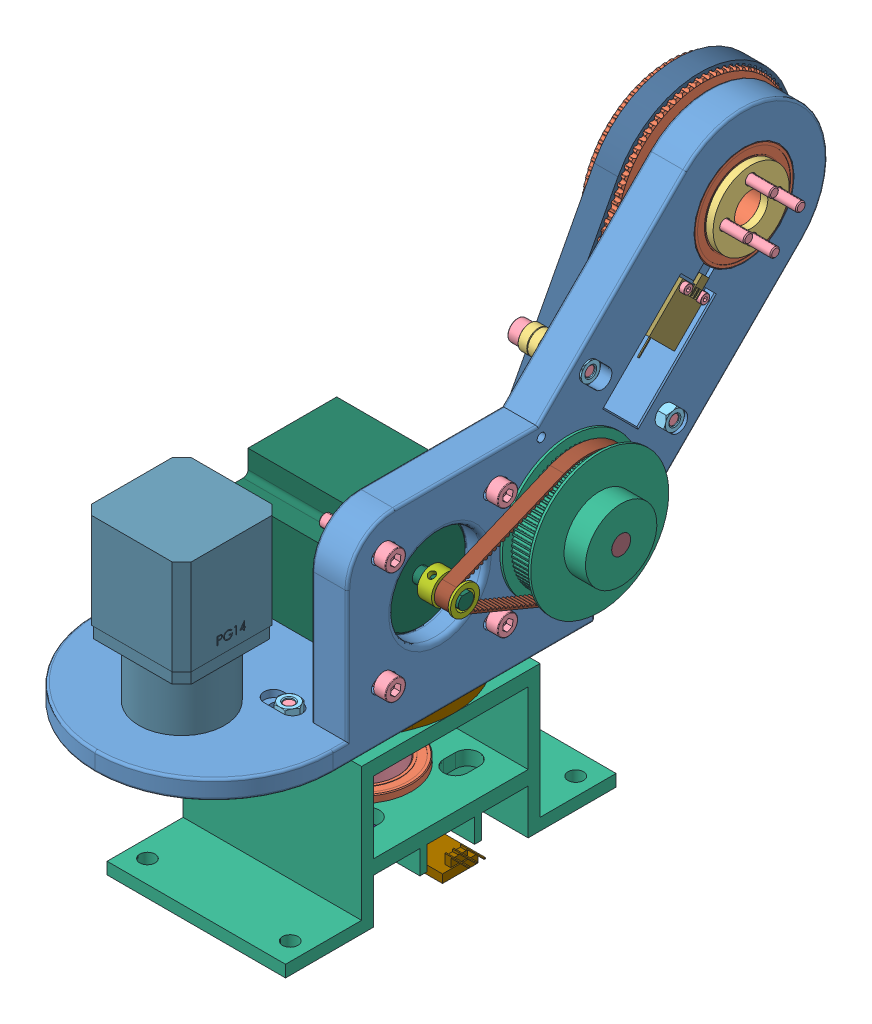
SolidWorks assembly arm1, configuration Default. Lengths in mm.
Overall size (123.1 252.71 277.96).
84 component instances, 27 part files, 181 mates.
Components (placement in the parent):
- arm1-1: arm1 [Default] at (0 22.25 32) x (0 0 1) z (0 1 0) size (257.74 100 155.28)
- PulleyHtd3m80Tbore8-2: PulleyHtd3m80Tbore8 [Default] at (25.5 142.4912 -110.7437) x (0 -0.999796 -0.020218) z (1 0 0) size (75.96 75.93 32)
- bearingCover-1: bearingCover [Default] at (50 142.4912 -110.7437) x (0 -0.999796 -0.020218) z (1 0 0) size (32 32 3)
- shaftJ1-1: shaftJ1 [Default] at (0 -34.75 0) x (0 0 -1) z (1 0 0) size (50 69 50)
- Pulleyhtd3m20Tbore8-1: Pulleyhtd3m20Tbore8 [Default] at (0 12.5 75.6) x (1 0 0) z (0 -1 0) size (22 22 24)
- pulley2GT80T-1: pulley2GT80T [Default] at (57.6 67.75 -36.0025) x (0 -0.778145 -0.628085) z (1 0 0) size (58 58 22)
- pulley2GT16Tbore6.35-1: pulley2GT16Tbore6.35 [Default] at (56.1 67.75 17.0975) x (0 0.483708 -0.87523) z (1 0 0) size (12.2 12.2 14)
- PulleyHTD3m15Tbore8-1: PulleyHTD3m15Tbore8 [Default] at (26.5 67.75 -36.0025) x (0 0.57686 0.816843) z (1 0 0) size (14 14 19.5)
- BeltHTD3m312L20T80T-1: BeltHTD3m312L20T80T [Default] at (0 12.5 0) x (0 0 1) z (0 1 0) size (125.04 78.09 10)
- BeltHTD3m363L15T80T-1: BeltHTD3m363L15T80T [Default] at (26.5 142.4912 -110.7437) x (0 -0.707107 0.707107) z (-1 0 0) size (152.76 78.09 10)
- belt2GT210L-1: belt2GT210L [Default] at (56.1 67.75 17.0975) x (0 0 -1) z (1 0 0) size (84.41 51.68 6)
- MagneticSensorV2-2: MagneticSensorV2 [Default] at (45.9 115.6211 -83.8737) x (0 -0.707107 0.707107) z (1 0 0) size (31 15 9)
- shaft8x70-1: shaft8x70 [Default] at (73.1 67.75 -36.0025) x (0 0 1) z (-1 0 0) size (8 8 61)
- Nema17L40PG14-1: Nema17L40PG14 [Default] at (0 99.75 75.6) x (0 0 -1) z (0 -1 0) size (42 42 88.5)
- Nema23_57x57x56-2: Nema23_57x57x56 [Default] at (-12 67.75 17.0975) x (0 0 -1) z (1 0 0) size (57 57 73)
- BeltTensionSpacer-1: BeltTensionSpacer [Default] at (35 113.7119 -46.6091) x (0 -0.41678 -0.909008) z (-1 0 0) size (6.4 6.4 3)
- BeltTensionSpacer-2: BeltTensionSpacer [Default] at (35 78.3566 -81.9645) x (0 -0.41678 -0.909008) z (-1 0 0) size (6.4 6.4 3)
- BeltTensionSpacer-6: BeltTensionSpacer [Default] at (-24.5 19.25 55) x (0.999608 0 0.027999) z (0 1 0) size (6.4 6.4 3)
- BeltTensionSpacer-5: BeltTensionSpacer [Default] at (24.5 22.25 55) x (0.852155 0 0.52329) z (0 -1 0) size (6.4 6.4 3)
- Washer45x60x1-2: Washer45x60x1 [5909K79] at (0 22.25 0) x (0 -1 0) z (0.730209 0 -0.683224) size (1 65 65)
- Washer45x60x1-1: Washer45x60x1 [5909K79] at (0 18.3 0) x (0 -1 0) z (0.528749 0 -0.848778) size (1 65 65)
- NeedleThrustBearing5909_45x60x3-1: NeedleThrustBearing5909_45x60x3 [5909K19] at (0 20.275 0) x (0.862783 0 0.505574) z (0.505574 0 -0.862783) size (65 3 65)
- bearing608 8x22x7-1: bearing608 8x22x7 [Default] at (50 67.75 -36.0025) x (0 -0.065699 -0.997839) z (0 0.997839 -0.065699) size (22 7 22)
- bearing608 8x22x7-2: bearing608 8x22x7 [Default] at (35 67.75 -36.0025) x (0 -0.995759 -0.092005) z (0 -0.092005 0.995759) size (22 7 22)
- bearing6806 30x42x7-3: bearing6806 30x42x7 [5972K282] at (38.5 142.4912 -110.7437) x (0 0.778145 0.628085) z (1 0 0) size (42 42 7)
- bearing6806 30x42x7-4: bearing6806 30x42x7 [5972K282] at (46.5 142.4912 -110.7437) x (0 -0.232241 -0.972658) z (-1 0 0) size (42 42 7)
- Bearing105 5x10x4-1: Bearing105 5x10x4 [7804K106] at (30 113.7119 -46.6091) x (0 0.558787 -0.829311) z (-1 0 0) size (10 10 4)
- Bearing105 5x10x4-4: Bearing105 5x10x4 [7804K106] at (26.1 78.3566 -81.9645) x (0 -0.623411 0.781894) z (-1 0 0) size (10 10 4)
- Bearing105 5x10x4-9: Bearing105 5x10x4 [7804K106] at (24.5 17.25 55) x (0.890608 0 -0.454771) z (0 -1 0) size (10 10 4)
- Bearing105 5x10x4-10: Bearing105 5x10x4 [7804K106] at (24.5 13.25 55) x (0.890608 0 -0.454771) z (0 -1 0) size (10 10 4)
- Bearing105 5x10x4-11: Bearing105 5x10x4 [7804K106] at (-24.5 13.25 55) x (-0.374722 0 0.927137) z (0 1 0) size (10 10 4)
- Bearing105 5x10x4-12: Bearing105 5x10x4 [7804K106] at (-24.5 17.25 55) x (0.156116 0 0.987739) z (0 1 0) size (10 10 4)
- Bearing105 5x10x4-2: Bearing105 5x10x4 [7804K106] at (26 113.7119 -46.6091) x (0 -0.774653 -0.632387) z (-1 0 0) size (10 10 4)
- Bearing105 5x10x4-3: Bearing105 5x10x4 [7804K106] at (30.1 78.3566 -81.9645) x (0 -0.931032 -0.364937) z (1 0 0) size (10 10 4)
- socket head cap screw_iso-13: socket head cap screw_iso [ISO 4762 M4 x 12 - 12N] at (0 38.25 20) x (0 -1 0) z (0 0 1) size (16 7 7)
- socket head cap screw_iso-14: socket head cap screw_iso [ISO 4762 M4 x 12 - 12N] at (20 38.25 0) x (0 -1 0) z (0 0 1) size (16 7 7)
- socket head cap screw_iso-15: socket head cap screw_iso [ISO 4762 M4 x 12 - 12N] at (0 38.25 -20) x (0 -1 0) z (0 0 1) size (16 7 7)
- socket head cap screw_iso-16: socket head cap screw_iso [ISO 4762 M4 x 12 - 12N] at (-20 38.25 0) x (0 -1 0) z (0 0 1) size (16 7 7)
- hex nut style 1 gradeab_iso-1: hex nut style 1 gradeab_iso [ISO - 4032 - M5 - W - N] at (49.7 113.7119 -46.6091) x (0 -0.707107 0.707107) z (1 0 0) size (8 9.24 4.7)
- hex nut style 1 gradeab_iso-2: hex nut style 1 gradeab_iso [ISO - 4032 - M5 - W - N] at (49.7 78.3566 -81.9645) x (0 0.965926 0.258819) z (1 0 0) size (8 9.24 4.7)
- socket head cap screw_iso-20: socket head cap screw_iso [ISO 4762 M5 x 25 - 25N] at (19 113.7119 -46.6091) size (30 8.5 8.5)
- socket head cap screw_iso-21: socket head cap screw_iso [ISO 4762 M5 x 25 - 25N] at (19.1 78.3566 -81.9645) size (30 8.5 8.5)
- socket head cap screw_iso-57: socket head cap screw_iso [ISO 4762 M5 x 20 - 20N] at (24.5 6.25 55) x (0 1 0) z (0 0 1) size (25 8.5 8.5)
- socket head cap screw_iso-58: socket head cap screw_iso [ISO 4762 M5 x 20 - 20N] at (-24.5 6.25 55) x (0 1 0) z (0 0 1) size (25 8.5 8.5)
- hex nut style 1 gradeab_iso-15: hex nut style 1 gradeab_iso [ISO - 4032 - M5 - W - N] at (-24.5 31.95 55) x (-0.866025 0 0.5) z (0 1 0) size (8 9.24 4.7)
- hex nut style 1 gradeab_iso-16: hex nut style 1 gradeab_iso [ISO - 4032 - M5 - W - N] at (24.5 31.95 55) x (-0.866025 0 -0.5) z (0 1 0) size (8 9.24 4.7)
- socket head cap screw_iso-63: socket head cap screw_iso [ISO 4762 M4 x 40 - 20N] at (19 153.4889 -110.5213) size (44 7 7)
- socket head cap screw_iso-64: socket head cap screw_iso [ISO 4762 M4 x 40 - 20N] at (19 142.7136 -121.7415) size (44 7 7)
- socket head cap screw_iso-65: socket head cap screw_iso [ISO 4762 M4 x 40 - 20N] at (19 131.4934 -110.9661) size (44 7 7)
- socket head cap screw_iso-66: socket head cap screw_iso [ISO 4762 M4 x 40 - 20N] at (19 142.2688 -99.746) size (44 7 7)
- socket head cap screw_iso-80: socket head cap screw_iso [ISO 4762 M2 x 12 - 12N] at (51.4 117.7424 -93.066) x (-1 0 0) z (0 0.924225 0.381849) size (14 3.8 3.8)
- socket head cap screw_iso-81: socket head cap screw_iso [ISO 4762 M2 x 12 - 12N] at (51.4 124.8135 -85.995) x (-1 0 0) z (0 0.924225 0.381849) size (14 3.8 3.8)
- hex nut style 1 gradeab_iso-25: hex nut style 1 gradeab_iso [ISO - 4032 - M2 - W - N] at (37.4 117.7424 -93.066) x (0 0 1) z (-1 0 0) size (4 4.62 1.6)
- hex nut style 1 gradeab_iso-26: hex nut style 1 gradeab_iso [ISO - 4032 - M2 - W - N] at (37.4 124.8135 -85.995) x (0 0 1) z (-1 0 0) size (4 4.62 1.6)
- socket head cap screw_iso-96: socket head cap screw_iso [ISO 4762 M5 x 25 - 25N] at (55 91.32 40.6675) x (-1 0 0) z (0 -0.924225 -0.381849) size (30 8.5 8.5)
- socket head cap screw_iso-97: socket head cap screw_iso [ISO 4762 M5 x 25 - 25N] at (55 91.32 -6.4725) x (-1 0 0) z (0 -0.924225 -0.381849) size (30 8.5 8.5)
- socket head cap screw_iso-98: socket head cap screw_iso [ISO 4762 M5 x 25 - 25N] at (55 44.18 -6.4725) x (-1 0 0) z (0 -0.924225 -0.381849) size (30 8.5 8.5)
- socket head cap screw_iso-99: socket head cap screw_iso [ISO 4762 M5 x 25 - 25N] at (55 44.18 40.6675) x (-1 0 0) z (0 -0.924225 -0.381849) size (30 8.5 8.5)
- socket head cap screw_iso-104: socket head cap screw_iso [ISO 4762 M3 x 12 - 12N] at (9.8995 19.25 85.4995) x (0 1 0) z (0 0 1) size (15 5.5 5.5)
- socket head cap screw_iso-105: socket head cap screw_iso [ISO 4762 M3 x 12 - 12N] at (9.8995 19.25 65.7005) x (0 1 0) z (0 0 1) size (15 5.5 5.5)
- socket head cap screw_iso-106: socket head cap screw_iso [ISO 4762 M3 x 12 - 12N] at (-9.8995 19.25 85.4995) x (0 1 0) z (0 0 1) size (15 5.5 5.5)
- socket head cap screw_iso-107: socket head cap screw_iso [ISO 4762 M3 x 12 - 12N] at (-9.8995 19.25 65.7005) x (0 1 0) z (0 0 1) size (15 5.5 5.5)
- hex nut style 1 gradeab_iso-35: hex nut style 1 gradeab_iso [ISO - 4032 - M5 - W - N] at (30.3 91.32 40.6675) x (0 0 1) z (-1 0 0) size (8 9.24 4.7)
- hex nut style 1 gradeab_iso-36: hex nut style 1 gradeab_iso [ISO - 4032 - M5 - W - N] at (30.3 91.32 -6.4725) x (0 0 1) z (-1 0 0) size (8 9.24 4.7)
- hex nut style 1 gradeab_iso-37: hex nut style 1 gradeab_iso [ISO - 4032 - M5 - W - N] at (30.3 44.18 -6.4725) x (0 0 1) z (-1 0 0) size (8 9.24 4.7)
- hex nut style 1 gradeab_iso-38: hex nut style 1 gradeab_iso [ISO - 4032 - M5 - W - N] at (40.3966 44.18 40.6675) x (0 0 -1) z (1 0 0) size (8 9.24 4.7)
- base-1: base [Default] x (1 0 0) z (0 1 0) size (75 138.93 61)
- bearing6806 30x42x7-1: bearing6806 30x42x7 [5972K282] at (0 -30.5984 0) x (0.837169 0 0.546944) z (0 -1 0) size (42 42 7)
- pulleyHTD3m80Tbase-1: pulleyHTD3m80Tbase [Default] at (0 12 0) x (1 0 0) z (0 1 0) size (75.63 75.63 12)
- bearing6806 30x42x7-2: bearing6806 30x42x7 [5972K282] at (0 14.3 0) x (0.999895 0 -0.014508) z (0 1 0) size (42 42 7)
- shaftJ1endPlate-1: shaftJ1endPlate [Default] at (0 -34.75 0) x (0 0 -1) z (0 -1 0) size (40 40 6)
- MagneticSensor-3: MagneticSensor [Default] at (31.5 -49.5984 0) x (1 0 0) z (0 1 0) size (31 15 7.5)
- socket head cap screw_iso-132: socket head cap screw_iso [ISO 4762 M5 x 16 - 16N] at (21 -5 -21) x (0 1 0) z (0 0 1) size (21 8.5 8.5)
- socket head cap screw_iso-133: socket head cap screw_iso [ISO 4762 M5 x 16 - 16N] at (21 -5 21) x (0 1 0) z (0 0 1) size (21 8.5 8.5)
- socket head cap screw_iso-134: socket head cap screw_iso [ISO 4762 M5 x 16 - 16N] at (-21 -5 21) x (0 1 0) z (0 0 1) size (21 8.5 8.5)
- socket head cap screw_iso-135: socket head cap screw_iso [ISO 4762 M5 x 16 - 16N] at (-21 -5 -21) x (0 1 0) z (0 0 1) size (21 8.5 8.5)
- socket head cap screw_iso-136: socket head cap screw_iso [ISO 4762 M3 x 16 - 16N] at (12.5 -43.75 0) x (0 1 0) z (0 0 1) size (19 5.5 5.5)
- socket head cap screw_iso-137: socket head cap screw_iso [ISO 4762 M3 x 16 - 16N] at (0 -43.75 12.5) x (0 1 0) z (0 0 1) size (19 5.5 5.5)
- socket head cap screw_iso-138: socket head cap screw_iso [ISO 4762 M3 x 16 - 16N] at (-12.5 -43.75 0) x (0 1 0) z (0 0 1) size (19 5.5 5.5)
- socket head cap screw_iso-139: socket head cap screw_iso [ISO 4762 M3 x 16 - 16N] at (0 -43.75 -12.5) x (0 1 0) z (0 0 1) size (19 5.5 5.5)
- socket head cap screw_iso-140: socket head cap screw_iso [ISO 4762 M2 x 12 - 12N] at (23.5 -51.5984 -5) x (0 1 0) z (-0.11823 0 0.992986) size (14 3.8 3.8)
- socket head cap screw_iso-141: socket head cap screw_iso [ISO 4762 M2 x 12 - 12N] at (23.5 -51.5984 5) x (0 1 0) z (0 0 1) size (14 3.8 3.8)
- hex nut style 1 gradeab_iso-59: hex nut style 1 gradeab_iso [ISO - 4032 - M2 - W - N] at (23.5 -40.9984 -5) x (1 0 0) z (0 1 0) size (4 4.62 1.6)
- hex nut style 1 gradeab_iso-60: hex nut style 1 gradeab_iso [ISO - 4032 - M2 - W - N] at (23.5 -40.9984 5) x (1 0 0) z (0 1 0) size (4 4.62 1.6)
Mates (geometry in assembly coordinates):
- Fix J1: parallel aligned: plane of base-1 through (37.5 6 37.5) normal (1 0 0); plane of arm1-1 through (50 30.25 -48) normal (1 0 0)
- Concentric1: concentric aligned: cylinder of base-1 through (0 29.44 0) axis (0 -1 0) radius 21.05; cylinder of bearing6806 30x42x7-1 through (0 -34.0984 0) axis (0 -1 0) radius 21
- Coincident1: coincident anti-aligned: plane of base-1 through (0 -34.0984 0) normal (0 1 0); plane of bearing6806 30x42x7-1 through (-11.2944 -34.0984 17.2875) normal (0 -1 0)
- Concentric2: concentric anti-aligned: cylinder of base-1 through (0 6 0) axis (0 -1 0) radius 16; cylinder of pulleyHTD3m80Tbase-1 through (0 10.8 0) axis (0 1 0) radius 21.05
- Concentric3: concentric anti-aligned: cylinder of base-1 through (21 6 21) axis (0 -1 0) radius 2.75; cylinder of pulleyHTD3m80Tbase-1 through (21 6 21) axis (0 1 0) radius 3
- Coincident2: coincident anti-aligned: plane of base-1 through (0 6 0) normal (0 1 0); plane of pulleyHTD3m80Tbase-1 through (0 6 0) normal (0 -1 0)
- Concentric4: concentric aligned: cylinder of base-1 through (21 6 -21) axis (0 -1 0) radius 2.75; cylinder of socket head cap screw_iso-132 through (21 -36.75 -21) axis (0 -1 0) radius 4.25
- Coincident3: coincident anti-aligned: plane of base-1 through (0 0 0) normal (0 -1 0); plane of socket head cap screw_iso-132 through (16.75 0 -21) normal (0 1 0)
- Concentric5: concentric aligned: cylinder of base-1 through (21 6 21) axis (0 -1 0) radius 2.75; cylinder of socket head cap screw_iso-133 through (21 -36.75 21) axis (0 -1 0) radius 4.25
- Coincident4: coincident anti-aligned: plane of base-1 through (0 0 0) normal (0 -1 0); plane of socket head cap screw_iso-133 through (16.75 0 21) normal (0 1 0)
- Concentric6: concentric aligned: cylinder of base-1 through (-21 6 21) axis (0 -1 0) radius 2.75; cylinder of socket head cap screw_iso-134 through (-21 -36.75 21) axis (0 -1 0) radius 4.25
- Coincident5: coincident anti-aligned: plane of base-1 through (0 0 0) normal (0 -1 0); plane of socket head cap screw_iso-134 through (-25.25 0 21) normal (0 1 0)
- Concentric7: concentric aligned: cylinder of base-1 through (-21 6 -21) axis (0 -1 0) radius 2.75; cylinder of socket head cap screw_iso-135 through (-21 -36.75 -21) axis (0 -1 0) radius 4.25
- Coincident6: coincident anti-aligned: plane of base-1 through (0 0 0) normal (0 -1 0); plane of socket head cap screw_iso-135 through (-25.25 0 -21) normal (0 1 0)
- Concentric8: concentric aligned: cylinder of pulleyHTD3m80Tbase-1 through (0 10.8 0) axis (0 1 0) radius 21.05; cylinder of bearing6806 30x42x7-2 through (0 17.8 0) axis (0 1 0) radius 21
- Coincident7: coincident anti-aligned: plane of pulleyHTD3m80Tbase-1 through (0 10.8 0) normal (0 1 0); plane of bearing6806 30x42x7-2 through (-0.2996 10.8 -20.6478) normal (0 -1 0)
- Concentric9: concentric aligned: cylinder of pulleyHTD3m80Tbase-1 through (0 10.8 0) axis (0 1 0) radius 21.05; cylinder of Washer45x60x1-1 through (0 17.8 0) axis (0 1 0) radius 32.5
- Coincident8: coincident anti-aligned: plane of pulleyHTD3m80Tbase-1 through (0 17.8 0) normal (0 1 0); plane of Washer45x60x1-1 through (0 17.8 0) normal (0 -1 0)
- Concentric10: concentric anti-aligned: cylinder of pulleyHTD3m80Tbase-1 through (0 10.8 0) axis (0 1 0) radius 21.05; cylinder of NeedleThrustBearing5909_45x60x3-1 through (0 18.775 0) axis (0 -1 0) radius 32.5
- Distance1: distance = 0.2 mm anti-aligned: plane of NeedleThrustBearing5909_45x60x3-1 through (-16.4311 19 28.0405) normal (0 -1 0); plane of Washer45x60x1-1 through (0 18.8 0) normal (0 1 0)
- Concentric11: concentric aligned: cylinder of pulleyHTD3m80Tbase-1 through (0 10.8 0) axis (0 1 0) radius 21.05; cylinder of Washer45x60x1-2 through (0 21.75 0) axis (0 1 0) radius 22.525
- Distance2: distance = 0.2 mm anti-aligned: plane of NeedleThrustBearing5909_45x60x3-1 through (-16.2626 21.55 27.7529) normal (0 1 0); plane of Washer45x60x1-2 through (0 21.75 0) normal (0 -1 0)
- Concentric12: concentric aligned: cylinder of base-1 through (0 6 0) axis (0 -1 0) radius 16; cylinder of arm1-1 through (0 30.25 0) axis (0 -1 0) radius 15.5
- Coincident12: coincident anti-aligned: plane of arm1-1 through (0 22.75 0) normal (0 -1 0); plane of Washer45x60x1-2 through (0 22.75 0) normal (0 1 0)
- Concentric15: concentric anti-aligned: cylinder of arm1-1 through (0 30.25 75.6) axis (0 -1 0) radius 11.5; cylinder of Nema17L40PG14-1 through (0 30.25 75.6) axis (0 1 0) radius 18
- Concentric16: concentric aligned: cylinder of arm1-1 through (-9.8995 30.25 85.4995) axis (0 -1 0) radius 1.65; cylinder of Nema17L40PG14-1 through (-9.8995 38.25 85.4995) axis (0 -1 0) radius 2
- Coincident16: coincident anti-aligned: plane of arm1-1 through (0 30.25 32) normal (0 1 0); plane of Nema17L40PG14-1 through (0 30.25 75.6) normal (0 -1 0)
- Concentric20: concentric anti-aligned: cylinder of Nema17L40PG14-1 through (0 11.25 75.6) axis (0 1 0) radius 4; cylinder of Pulleyhtd3m20Tbore8-1 through (0 30 75.6) axis (0 -1 0) radius 11
- Coincident17: coincident anti-aligned: plane of pulleyHTD3m80Tbase-1 through (0 18 0) normal (0 1 0); plane of Pulleyhtd3m20Tbore8-1 through (0 18 75.6) normal (0 -1 0)
- Concentric21: concentric aligned: cylinder of NeedleThrustBearing5909_45x60x3-1 through (0 18.775 0) axis (0 -1 0) radius 32.5; cylinder of BeltHTD3m312L20T80T-1 through (0 17.5 0) axis (0 -1 0) radius 39.0462
- Concentric22: concentric aligned: cylinder of Pulleyhtd3m20Tbore8-1 through (0 30 75.6) axis (0 -1 0) radius 11; cylinder of BeltHTD3m312L20T80T-1 through (0 17.5 75.6) axis (0 -1 0) radius 10.3983
- Distance3: distance = 0.5 mm anti-aligned: plane of Pulleyhtd3m20Tbore8-1 through (0 18 75.6) normal (0 -1 0); plane of BeltHTD3m312L20T80T-1 through (0 17.5 0) normal (0 1 0)
- Concentric23: concentric aligned: cylinder of arm1-1 through (0 30.25 0) axis (0 -1 0) radius 15.5; cylinder of shaftJ1-1 through (0 30.25 0) axis (0 -1 0) radius 15
- Concentric24: concentric aligned: cylinder of arm1-1 through (0 30.25 20) axis (0 -1 0) radius 2.75; cylinder of shaftJ1-1 through (0 34.25 20) axis (0 -1 0) radius 2.25
- Coincident19: coincident anti-aligned: plane of arm1-1 through (0 30.25 32) normal (0 1 0); plane of shaftJ1-1 through (0 30.25 0) normal (0 -1 0)
- Coincident24: coincident anti-aligned: plane of shaftJ1-1 through (0 -34.75 0) normal (0 -1 0); plane of shaftJ1endPlate-1 through (0 -34.75 0) normal (0 1 0)
- Concentric29: concentric anti-aligned: cylinder of shaftJ1-1 through (0 -14.75 12.5) axis (0 -1 0) radius 1.4; cylinder of shaftJ1endPlate-1 through (0 -40.75 12.5) axis (0 1 0) radius 1.75
- Concentric36: concentric anti-aligned: cylinder of shaftJ1-1 through (0 34.25 20) axis (0 -1 0) radius 2.25; cylinder of socket head cap screw_iso-13 through (0 70 20) axis (0 1 0) radius 3.5
- Coincident31: coincident anti-aligned: plane of shaftJ1-1 through (0 34.25 0) normal (0 1 0); plane of socket head cap screw_iso-13 through (3.5 34.25 20) normal (0 -1 0)
- Concentric37: concentric anti-aligned: cylinder of shaftJ1-1 through (20 34.25 0) axis (0 -1 0) radius 2.25; cylinder of socket head cap screw_iso-14 through (20 70 0) axis (0 1 0) radius 3.5
- Coincident32: coincident anti-aligned: plane of shaftJ1-1 through (0 34.25 0) normal (0 1 0); plane of socket head cap screw_iso-14 through (23.5 34.25 0) normal (0 -1 0)
- Concentric38: concentric anti-aligned: cylinder of shaftJ1-1 through (0 34.25 -20) axis (0 -1 0) radius 2.25; cylinder of socket head cap screw_iso-15 through (0 70 -20) axis (0 1 0) radius 3.5
- Coincident33: coincident anti-aligned: plane of shaftJ1-1 through (0 34.25 0) normal (0 1 0); plane of socket head cap screw_iso-15 through (3.5 34.25 -20) normal (0 -1 0)
- Concentric39: concentric anti-aligned: cylinder of shaftJ1-1 through (-20 34.25 0) axis (0 -1 0) radius 2.25; cylinder of socket head cap screw_iso-16 through (-20 70 0) axis (0 1 0) radius 3.5
- Coincident34: coincident anti-aligned: circle of shaftJ1-1; plane of socket head cap screw_iso-16 through (-16.5 34.25 0) normal (0 -1 0)
- Concentric41: concentric anti-aligned: cylinder of arm1-1 through (35 67.75 17.0975) axis (1 0 0) radius 19.5; cylinder of Nema23_57x57x56-2 through (61 67.75 17.0975) axis (-1 0 0) radius 3.175
- Coincident36: coincident anti-aligned: plane of arm1-1 through (40 22.25 32) normal (-1 0 0); plane of Nema23_57x57x56-2 through (40 67.75 17.0975) normal (1 0 0)
- Parallel2: parallel aligned: plane of arm1-1 through (35 105.25 55.9949) normal (0 1 0); plane of Nema23_57x57x56-2 through (40 96.25 45.5975) normal (0 1 0)
- Concentric42: concentric anti-aligned: cylinder of pulley2GT16Tbore6.35-1 through (46.6 67.75 17.0975) axis (1 0 0) radius 6.1; cylinder of Nema23_57x57x56-2 through (61 67.75 17.0975) axis (-1 0 0) radius 3.175
- Concentric43: concentric aligned: cylinder of arm1-1 through (43 67.75 -36.0025) axis (1 0 0) radius 11.05; cylinder of bearing608 8x22x7-1 through (43 67.75 -36.0025) axis (1 0 0) radius 11
- Coincident41: coincident anti-aligned: plane of arm1-1 through (43 67.75 -36.0025) normal (1 0 0); plane of bearing608 8x22x7-1 through (43 67.75 -36.0025) normal (-1 0 0)
- Concentric44: concentric aligned: cylinder of arm1-1 through (42 67.75 -36.0025) axis (-1 0 0) radius 11.05; cylinder of bearing608 8x22x7-2 through (42 67.75 -36.0025) axis (-1 0 0) radius 11
- Coincident42: coincident anti-aligned: plane of arm1-1 through (42 67.75 -36.0025) normal (-1 0 0); plane of bearing608 8x22x7-2 through (42 67.75 -36.0025) normal (1 0 0)
- Concentric45: concentric anti-aligned: cylinder of arm1-1 through (43 142.4912 -110.7437) axis (1 0 0) radius 21.05; cylinder of bearing6806 30x42x7-4 through (43 142.4912 -110.7437) axis (-1 0 0) radius 21
- Coincident43: coincident anti-aligned: plane of arm1-1 through (43 142.4912 -110.7437) normal (1 0 0); plane of bearing6806 30x42x7-4 through (43 122.4058 -105.9479) normal (-1 0 0)
- Concentric46: concentric anti-aligned: cylinder of arm1-1 through (42 142.4912 -110.7437) axis (-1 0 0) radius 21.05; cylinder of bearing6806 30x42x7-3 through (42 142.4912 -110.7437) axis (1 0 0) radius 21
- Coincident44: coincident anti-aligned: plane of arm1-1 through (42 142.4912 -110.7437) normal (-1 0 0); plane of bearing6806 30x42x7-3 through (42 129.5212 -94.675) normal (1 0 0)
- Concentric47: concentric aligned: cylinder of bearing608 8x22x7-1 through (43 67.75 -36.0025) axis (1 0 0) radius 4; cylinder of pulley2GT80T-1 through (51.1 67.75 -36.0025) axis (1 0 0) radius 4
- Distance4: distance = 0.5 mm aligned: plane of pulley2GT16Tbore6.35-1 through (52.6 67.75 17.0975) normal (1 0 0); plane of pulley2GT80T-1 through (52.1 67.75 -36.0025) normal (1 0 0)
- Concentric48: concentric anti-aligned: cylinder of bearing608 8x22x7-2 through (42 67.75 -36.0025) axis (-1 0 0) radius 4; cylinder of shaft8x70-1 through (12.1 67.75 -36.0025) axis (1 0 0) radius 4
- Coincident46: coincident aligned: plane of pulley2GT80T-1 through (73.1 67.75 -36.0025) normal (1 0 0); plane of shaft8x70-1 through (73.1 67.75 -36.0025) normal (1 0 0)
- disPulley1J1: distance = 5 mm anti-aligned: plane of pulley2GT16Tbore6.35-1 through (46.6 67.75 17.0975) normal (-1 0 0); plane of Nema23_57x57x56-2 through (41.6 67.75 17.0975) normal (1 0 0)
- Concentric51: concentric aligned: cylinder of pulley2GT80T-1 through (73.1 67.75 -36.0025) axis (-1 0 0) radius 15; cylinder of belt2GT210L-1 through (59.1 67.75 -36.0025) axis (-1 0 0) radius 25.84
- Concentric52: concentric anti-aligned: cylinder of pulley2GT16Tbore6.35-1 through (46.6 67.75 17.0975) axis (1 0 0) radius 6.1; cylinder of belt2GT210L-1 through (59.1 67.75 17.0975) axis (-1 0 0) radius 5.47
- Distance6: distance = 0.5 mm anti-aligned: plane of pulley2GT16Tbore6.35-1 through (52.6 67.75 17.0975) normal (1 0 0); plane of belt2GT210L-1 through (53.1 67.75 -36.0025) normal (-1 0 0)
- Concentric58: concentric aligned: cylinder of arm1-1 through (35 113.7119 -46.6091) axis (1 0 0) radius 2.75; cylinder of hex nut style 1 gradeab_iso-1 through (24.6625 113.7119 -46.6091) axis (1 0 0) radius 2.5
- Coincident53: coincident anti-aligned: plane of arm1-1 through (45 114.7726 -45.5485) normal (1 0 0); plane of hex nut style 1 gradeab_iso-1 through (45 119.3688 -52.266) normal (-1 0 0)
- Coincident54: coincident anti-aligned: plane of arm1-1 through (45 117.601 -48.3769) normal (0 -0.707107 0.707107); plane of hex nut style 1 gradeab_iso-1 through (45 114.9074 -51.0705) normal (0 0.707107 -0.707107)
- Concentric591: concentric aligned: cylinder of arm1-1 through (35 78.3566 -81.9645) axis (1 0 0) radius 2.75; cylinder of hex nut style 1 gradeab_iso-2 through (24.6625 78.3566 -81.9645) axis (1 0 0) radius 2.5
- Coincident551: coincident anti-aligned: plane of arm1-1 through (45 82.9528 -77.3683) normal (1 0 0); plane of hex nut style 1 gradeab_iso-2 through (45 70.6292 -84.035) normal (-1 0 0)
- Coincident56: coincident anti-aligned: plane of arm1-1 through (45 85.7812 -80.1967) normal (0 -0.707107 0.707107); plane of hex nut style 1 gradeab_iso-2 through (45 79.552 -86.4259) normal (0 0.707107 -0.707107)
- Concentric60: concentric anti-aligned: cylinder of arm1-1 through (35 113.7119 -46.6091) axis (1 0 0) radius 2.75; cylinder of Bearing105 5x10x4-1 through (28 113.7119 -46.6091) axis (-1 0 0) radius 5
- Distance8: distance = 3 mm anti-aligned: plane of arm1-1 through (35 142.4912 -110.7437) normal (-1 0 0); plane of Bearing105 5x10x4-1 through (32 109.7312 -49.2913) normal (1 0 0)
- Concentric61: concentric aligned: cylinder of Bearing105 5x10x4-1 through (28 113.7119 -46.6091) axis (-1 0 0) radius 5; cylinder of Bearing105 5x10x4-2 through (24 113.7119 -46.6091) axis (-1 0 0) radius 5
- Coincident58: coincident anti-aligned: plane of Bearing105 5x10x4-1 through (28 109.7312 -49.2913) normal (-1 0 0); plane of Bearing105 5x10x4-2 through (28 110.6765 -42.8908) normal (1 0 0)
- Concentric63: concentric aligned: cylinder of Bearing105 5x10x4-2 through (24 113.7119 -46.6091) axis (-1 0 0) radius 3.4863; cylinder of socket head cap screw_iso-20 through (-12.75 113.7119 -46.6091) axis (-1 0 0) radius 4.25
- Coincident60: coincident anti-aligned: plane of Bearing105 5x10x4-2 through (24 111.5073 -43.9085) normal (-1 0 0); plane of socket head cap screw_iso-20 through (24 117.9619 -46.6091) normal (1 0 0)
- Concentric64: concentric anti-aligned: cylinder of socket head cap screw_iso-20 through (-12.75 113.7119 -46.6091) axis (-1 0 0) radius 2.5; cylinder of BeltTensionSpacer-1 through (32 113.7119 -46.6091) axis (1 0 0) radius 3.2
- Coincident61: coincident anti-aligned: plane of arm1-1 through (35 142.4912 -110.7437) normal (-1 0 0); plane of BeltTensionSpacer-1 through (35 113.7119 -46.6091) normal (1 0 0)
- Concentric65: concentric aligned: cylinder of arm1-1 through (35 78.3566 -81.9645) axis (1 0 0) radius 2.75; cylinder of BeltTensionSpacer-2 through (32 78.3566 -81.9645) axis (1 0 0) radius 3.2
- Coincident62: coincident aligned: plane of arm1-1 through (35 142.4912 -110.7437) normal (-1 0 0); circle of BeltTensionSpacer-2
- Concentric66: concentric aligned: cylinder of Bearing105 5x10x4-3 through (32.1 78.3566 -81.9645) axis (1 0 0) radius 5; cylinder of BeltTensionSpacer-2 through (32 78.3566 -81.9645) axis (1 0 0) radius 3.2
- Coincident63: coincident anti-aligned: plane of Bearing105 5x10x4-3 through (32 79.8214 -85.7014) normal (1 0 0); plane of BeltTensionSpacer-2 through (32 78.3566 -81.9645) normal (-1 0 0)
- Coincident64: coincident anti-aligned: plane of Bearing105 5x10x4-3 through (28.1 80.1083 -86.4334) normal (-1 0 0); plane of Bearing105 5x10x4-4 through (28.1 82.1097 -78.9721) normal (1 0 0)
- Concentric67: concentric anti-aligned: cylinder of Bearing105 5x10x4-3 through (32.1 78.3566 -81.9645) axis (1 0 0) radius 5; cylinder of Bearing105 5x10x4-4 through (24.1 78.3566 -81.9645) axis (-1 0 0) radius 5
- Concentric681: concentric aligned: cylinder of Bearing105 5x10x4-4 through (24.1 78.3566 -81.9645) axis (-1 0 0) radius 4.0137; cylinder of socket head cap screw_iso-21 through (-12.65 78.3566 -81.9645) axis (-1 0 0) radius 4.25
- Coincident651: coincident anti-aligned: plane of Bearing105 5x10x4-4 through (24.1 82.1097 -78.9721) normal (-1 0 0); plane of socket head cap screw_iso-21 through (24.1 82.6066 -81.9645) normal (1 0 0)
- Concentric786: concentric anti-aligned: cylinder of base-1 through (23.5 -46.0984 5) axis (0 1 0) radius 1.25; cylinder of MagneticSensor-3 through (23.5 -42.0984 5) axis (0 -1 0) radius 1.25
- Concentric787: concentric anti-aligned: cylinder of base-1 through (23.5 -46.0984 -5) axis (0 1 0) radius 1.25; cylinder of MagneticSensor-3 through (23.5 -42.0984 -5) axis (0 -1 0) radius 1.25
- Coincident749: coincident anti-aligned: plane of base-1 through (0 -46.0984 0) normal (0 -1 0); plane of MagneticSensor-3 through (31.5 -46.0984 0) normal (0 1 0)
- Coincident751: coincident anti-aligned: plane of arm1-1 through (45.9 22.25 32) normal (1 0 0); plane of MagneticSensorV2-2 through (45.9 115.6211 -83.8737) normal (-1 0 0)
- Concentric790: concentric anti-aligned: cylinder of arm1-1 through (35 117.7424 -93.066) axis (1 0 0) radius 1.25; cylinder of MagneticSensorV2-2 through (50.9 117.7424 -93.066) axis (-1 0 0) radius 1.25
- Concentric791: concentric anti-aligned: cylinder of arm1-1 through (35 124.8135 -85.995) axis (1 0 0) radius 1.25; cylinder of MagneticSensorV2-2 through (50.9 124.8135 -85.995) axis (-1 0 0) radius 1.25
- Concentric7962: concentric aligned: cylinder of shaft8x70-1 through (12.1 67.75 -36.0025) axis (1 0 0) radius 4; cylinder of PulleyHTD3m15Tbore8-1 through (13.5 67.75 -36.0025) axis (1 0 0) radius 7
- Concentric7963: concentric anti-aligned: cylinder of shaftJ1endPlate-1 through (12.5 -40.75 0) axis (0 1 0) radius 1.75; cylinder of socket head cap screw_iso-136 through (12.5 -75.5 0) axis (0 -1 0) radius 2.75
- Coincident7532: coincident anti-aligned: plane of shaftJ1endPlate-1 through (0 -40.75 0) normal (0 -1 0); plane of socket head cap screw_iso-136 through (9.75 -40.75 0) normal (0 1 0)
- Concentric7964: concentric anti-aligned: cylinder of shaftJ1endPlate-1 through (0 -40.75 12.5) axis (0 1 0) radius 1.75; cylinder of socket head cap screw_iso-137 through (0 -75.5 12.5) axis (0 -1 0) radius 2.75
- Coincident7533: coincident anti-aligned: plane of shaftJ1endPlate-1 through (0 -40.75 0) normal (0 -1 0); plane of socket head cap screw_iso-137 through (-2.75 -40.75 12.5) normal (0 1 0)
- Concentric7965: concentric anti-aligned: cylinder of shaftJ1endPlate-1 through (-12.5 -40.75 0) axis (0 1 0) radius 1.75; cylinder of socket head cap screw_iso-138 through (-12.5 -75.5 0) axis (0 -1 0) radius 2.75
- Coincident7534: coincident anti-aligned: plane of shaftJ1endPlate-1 through (0 -40.75 0) normal (0 -1 0); plane of socket head cap screw_iso-138 through (-15.25 -40.75 0) normal (0 1 0)
- Concentric7966: concentric anti-aligned: cylinder of shaftJ1endPlate-1 through (0 -40.75 -12.5) axis (0 1 0) radius 1.75; cylinder of socket head cap screw_iso-139 through (0 -75.5 -12.5) axis (0 -1 0) radius 2.75
- Coincident7535: coincident anti-aligned: plane of shaftJ1endPlate-1 through (0 -40.75 0) normal (0 -1 0); plane of socket head cap screw_iso-139 through (-2.75 -40.75 -12.5) normal (0 1 0)
- Concentric7967: concentric aligned: cylinder of shaftJ1-1 through (0 30.25 0) axis (0 -1 0) radius 15; cylinder of shaftJ1endPlate-1 through (0 -35.75 0) axis (0 -1 0) radius 20
- Distance21: distance = 2 mm anti-aligned: plane of PulleyHTD3m15Tbore8-1 through (33 67.75 -36.0025) normal (1 0 0); plane of arm1-1 through (35 142.4912 -110.7437) normal (-1 0 0)
- Distance22: distance = 0.5 mm anti-aligned: plane of PulleyHTD3m15Tbore8-1 through (21 67.75 -36.0025) normal (1 0 0); plane of BeltHTD3m363L15T80T-1 through (21.5 142.4912 -110.7437) normal (-1 0 0)
- Concentric7968: concentric anti-aligned: cylinder of arm1-1 through (35 142.4912 -110.7437) axis (1 0 0) radius 35; cylinder of PulleyHtd3m80Tbore8-2 through (50 142.4912 -110.7437) axis (-1 0 0) radius 15
- Coincident7539: coincident anti-aligned: plane of arm1-1 through (35 142.4912 -110.7437) normal (-1 0 0); plane of PulleyHtd3m80Tbore8-2 through (35 142.4912 -110.7437) normal (1 0 0)
- Concentric7969: concentric anti-aligned: cylinder of PulleyHtd3m80Tbore8-2 through (18 142.4912 -110.7437) axis (1 0 0) radius 7; cylinder of bearingCover-1 through (53 142.4912 -110.7437) axis (-1 0 0) radius 7
- Coincident7540: coincident anti-aligned: plane of PulleyHtd3m80Tbore8-2 through (50 142.4912 -110.7437) normal (1 0 0); plane of bearingCover-1 through (50 142.4912 -110.7437) normal (-1 0 0)
- Concentric7970: concentric anti-aligned: cylinder of PulleyHtd3m80Tbore8-2 through (18 131.4934 -110.9661) axis (1 0 0) radius 2.25; cylinder of bearingCover-1 through (53 131.4934 -110.9661) axis (-1 0 0) radius 2.25
- Concentric7973: concentric aligned: cylinder of BeltHTD3m363L15T80T-1 through (21.5 142.4912 -110.7437) axis (1 0 0) radius 39.0462; cylinder of PulleyHtd3m80Tbore8-2 through (18 142.4912 -110.7437) axis (1 0 0) radius 7
- Concentric7974: concentric aligned: cylinder of shaft8x70-1 through (12.1 67.75 -36.0025) axis (1 0 0) radius 4; cylinder of BeltHTD3m363L15T80T-1 through (21.5 67.75 -36.0025) axis (1 0 0) radius 8.011
- Concentric7985: concentric anti-aligned: cylinder of arm1-1 through (24.5 177.4912 55) axis (0 -1 0) radius 2.75; cylinder of BeltTensionSpacer-5 through (24.5 19.25 55) axis (0 1 0) radius 3.2
- Coincident7549: coincident anti-aligned: plane of arm1-1 through (0 22.25 32) normal (0 -1 0); plane of BeltTensionSpacer-5 through (24.5 22.25 55) normal (0 1 0)
- Concentric7986: concentric anti-aligned: cylinder of BeltTensionSpacer-5 through (24.5 19.25 55) axis (0 1 0) radius 3.2; cylinder of Bearing105 5x10x4-9 through (24.5 15.25 55) axis (0 -1 0) radius 5
- Coincident7550: coincident anti-aligned: plane of BeltTensionSpacer-5 through (24.5 19.25 55) normal (0 -1 0); plane of Bearing105 5x10x4-9 through (26.6829 19.25 59.2749) normal (0 1 0)
- Coincident7551: coincident anti-aligned: plane of Bearing105 5x10x4-9 through (26.6829 15.25 59.2749) normal (0 -1 0); plane of Bearing105 5x10x4-10 through (26.6829 15.25 59.2749) normal (0 1 0)
- Concentric7987: concentric aligned: cylinder of Bearing105 5x10x4-9 through (24.5 15.25 55) axis (0 -1 0) radius 5; cylinder of Bearing105 5x10x4-10 through (24.5 11.25 55) axis (0 -1 0) radius 5
- Concentric7988: concentric aligned: cylinder of arm1-1 through (-24.5 177.4912 55) axis (0 -1 0) radius 2.75; cylinder of BeltTensionSpacer-6 through (-24.5 22.25 55) axis (0 -1 0) radius 3.2
- Coincident7552: coincident anti-aligned: plane of arm1-1 through (0 22.25 32) normal (0 -1 0); plane of BeltTensionSpacer-6 through (-24.5 22.25 55) normal (0 1 0)
- Concentric7989: concentric anti-aligned: cylinder of BeltTensionSpacer-6 through (-24.5 22.25 55) axis (0 -1 0) radius 3.2; cylinder of Bearing105 5x10x4-12 through (-24.5 19.25 55) axis (0 1 0) radius 5
- Coincident7553: coincident anti-aligned: plane of BeltTensionSpacer-6 through (-24.5 19.25 55) normal (0 -1 0); plane of Bearing105 5x10x4-12 through (-19.7589 19.25 54.2506) normal (0 1 0)
- Concentric7990: concentric aligned: cylinder of Bearing105 5x10x4-11 through (-24.5 15.25 55) axis (0 1 0) radius 5; cylinder of Bearing105 5x10x4-12 through (-24.5 19.25 55) axis (0 1 0) radius 5
- Coincident7554: coincident anti-aligned: plane of Bearing105 5x10x4-11 through (-20.0497 15.25 56.7987) normal (0 1 0); plane of Bearing105 5x10x4-12 through (-19.7589 15.25 54.2506) normal (0 -1 0)
- Concentric7991: concentric aligned: cylinder of Bearing105 5x10x4-10 through (24.5 11.25 55) axis (0 -1 0) radius 3.4863; cylinder of socket head cap screw_iso-57 through (24.5 -25.5 55) axis (0 -1 0) radius 4.25
- Coincident7555: coincident anti-aligned: plane of Bearing105 5x10x4-10 through (26.0855 11.25 58.1049) normal (0 -1 0); plane of socket head cap screw_iso-57 through (20.25 11.25 55) normal (0 1 0)
- Concentric7992: concentric anti-aligned: cylinder of Bearing105 5x10x4-11 through (-24.5 15.25 55) axis (0 1 0) radius 3.4863; cylinder of socket head cap screw_iso-58 through (-24.5 -25.5 55) axis (0 -1 0) radius 4.25
- Coincident7556: coincident anti-aligned: plane of Bearing105 5x10x4-11 through (-21.9967 11.25 56.0117) normal (0 -1 0); plane of socket head cap screw_iso-58 through (-28.75 11.25 55) normal (0 1 0)
- Concentric7994: concentric anti-aligned: cylinder of arm1-1 through (-24.5 177.4912 55) axis (0 -1 0) radius 2.75; cylinder of hex nut style 1 gradeab_iso-15 through (-24.5 6.9125 55) axis (0 1 0) radius 2.5
- Coincident7558: coincident anti-aligned: plane of arm1-1 through (-26 27.25 55) normal (0 1 0); plane of hex nut style 1 gradeab_iso-15 through (-17.5718 27.25 51) normal (0 -1 0)
- Concentric7995: concentric anti-aligned: cylinder of arm1-1 through (24.5 177.4912 55) axis (0 -1 0) radius 2.75; cylinder of hex nut style 1 gradeab_iso-16 through (24.5 6.9125 55) axis (0 1 0) radius 2.5
- Coincident7559: coincident anti-aligned: plane of arm1-1 through (18 27.25 55) normal (0 1 0); plane of hex nut style 1 gradeab_iso-16 through (31.4282 27.25 59) normal (0 -1 0)
- Coincident7560: coincident anti-aligned: plane of arm1-1 through (18 27.25 51) normal (0 0 1); plane of hex nut style 1 gradeab_iso-16 through (26.8094 27.25 51) normal (0 0 -1)
- Coincident7561: coincident anti-aligned: plane of arm1-1 through (-26 27.25 51) normal (0 0 1); plane of hex nut style 1 gradeab_iso-15 through (-22.1906 27.25 51) normal (0 0 -1)
- Concentric8000: concentric anti-aligned: cylinder of PulleyHtd3m80Tbore8-2 through (18 153.4889 -110.5213) axis (1 0 0) radius 2.25; cylinder of socket head cap screw_iso-63 through (-12.75 153.4889 -110.5213) axis (-1 0 0) radius 3.5
- Coincident7570: coincident anti-aligned: plane of PulleyHtd3m80Tbore8-2 through (23 153.4889 -110.5213) normal (-1 0 0); plane of socket head cap screw_iso-63 through (23 156.9889 -110.5213) normal (1 0 0)
- Concentric8001: concentric anti-aligned: cylinder of PulleyHtd3m80Tbore8-2 through (18 142.7136 -121.7415) axis (1 0 0) radius 2.25; cylinder of socket head cap screw_iso-64 through (-12.75 142.7136 -121.7415) axis (-1 0 0) radius 3.5
- Coincident7571: coincident anti-aligned: plane of PulleyHtd3m80Tbore8-2 through (23 142.7136 -121.7415) normal (-1 0 0); plane of socket head cap screw_iso-64 through (23 146.2136 -121.7415) normal (1 0 0)
- Concentric8002: concentric aligned: cylinder of PulleyHtd3m80Tbore8-2 through (23 131.4934 -110.9661) axis (-1 0 0) radius 3.6; cylinder of socket head cap screw_iso-65 through (-12.75 131.4934 -110.9661) axis (-1 0 0) radius 3.5
- Coincident7572: coincident anti-aligned: plane of PulleyHtd3m80Tbore8-2 through (23 131.4934 -110.9661) normal (-1 0 0); plane of socket head cap screw_iso-65 through (23 134.9934 -110.9661) normal (1 0 0)
- Concentric8003: concentric anti-aligned: cylinder of PulleyHtd3m80Tbore8-2 through (18 142.2688 -99.746) axis (1 0 0) radius 2.25; cylinder of socket head cap screw_iso-66 through (-12.75 142.2688 -99.746) axis (-1 0 0) radius 3.5
- Coincident7573: coincident anti-aligned: plane of PulleyHtd3m80Tbore8-2 through (23 142.2688 -99.746) normal (-1 0 0); plane of socket head cap screw_iso-66 through (23 145.7688 -99.746) normal (1 0 0)
- Concentric8033: concentric anti-aligned: cylinder of MagneticSensorV2-2 through (50.9 117.7424 -93.066) axis (-1 0 0) radius 1.25; cylinder of socket head cap screw_iso-80 through (83.15 117.7424 -93.066) axis (1 0 0) radius 1.9
- Coincident7610: coincident anti-aligned: plane of MagneticSensorV2-2 through (49.4 115.6211 -83.8737) normal (1 0 0); plane of socket head cap screw_iso-80 through (49.4 117.0169 -91.31) normal (-1 0 0)
- Concentric8034: concentric anti-aligned: cylinder of MagneticSensorV2-2 through (50.9 124.8135 -85.995) axis (-1 0 0) radius 1.25; cylinder of socket head cap screw_iso-81 through (83.15 124.8135 -85.995) axis (1 0 0) radius 1.9
- Coincident7611: coincident anti-aligned: plane of MagneticSensorV2-2 through (49.4 115.6211 -83.8737) normal (1 0 0); plane of socket head cap screw_iso-81 through (49.4 124.088 -84.2389) normal (-1 0 0)
- Concentric8035: concentric aligned: cylinder of MagneticSensor-3 through (23.5 -42.0984 -5) axis (0 -1 0) radius 1.25; cylinder of socket head cap screw_iso-140 through (23.5 -83.3484 -5) axis (0 -1 0) radius 1.9
- Concentric8036: concentric aligned: cylinder of MagneticSensor-3 through (23.5 -42.0984 5) axis (0 -1 0) radius 1.25; cylinder of socket head cap screw_iso-141 through (23.5 -83.3484 5) axis (0 -1 0) radius 1.9
- Coincident7612: coincident anti-aligned: plane of MagneticSensor-3 through (31.5 -49.5984 0) normal (0 -1 0); plane of socket head cap screw_iso-141 through (21.6 -49.5984 5) normal (0 1 0)
- Concentric8037: concentric aligned: cylinder of base-1 through (23.5 -46.0984 -5) axis (0 1 0) radius 1.25; cylinder of hex nut style 1 gradeab_iso-59 through (23.5 -66.0359 -5) axis (0 1 0) radius 1
- Coincident7613: coincident anti-aligned: plane of base-1 through (31 -42.5984 13) normal (0 1 0); plane of hex nut style 1 gradeab_iso-59 through (23.5 -42.5984 -7.3094) normal (0 -1 0)
- Concentric8038: concentric aligned: cylinder of base-1 through (23.5 -46.0984 5) axis (0 1 0) radius 1.25; cylinder of hex nut style 1 gradeab_iso-60 through (23.5 -66.0359 5) axis (0 1 0) radius 1
- Coincident7614: coincident anti-aligned: plane of base-1 through (31 -42.5984 13) normal (0 1 0); plane of hex nut style 1 gradeab_iso-60 through (23.5 -42.5984 2.6906) normal (0 -1 0)
- Concentric8039: concentric anti-aligned: cylinder of arm1-1 through (35 117.7424 -93.066) axis (1 0 0) radius 1.25; cylinder of hex nut style 1 gradeab_iso-25 through (62.4375 117.7424 -93.066) axis (-1 0 0) radius 1
- Coincident7615: coincident anti-aligned: plane of arm1-1 through (39 22.25 32) normal (-1 0 0); plane of hex nut style 1 gradeab_iso-25 through (39 120.0519 -93.066) normal (1 0 0)
- Concentric8040: concentric anti-aligned: cylinder of arm1-1 through (35 124.8135 -85.995) axis (1 0 0) radius 1.25; cylinder of hex nut style 1 gradeab_iso-26 through (62.4375 124.8135 -85.995) axis (-1 0 0) radius 1
- Coincident7616: coincident anti-aligned: plane of arm1-1 through (39 22.25 32) normal (-1 0 0); plane of hex nut style 1 gradeab_iso-26 through (39 127.1229 -85.995) normal (1 0 0)
- Concentric8058: concentric aligned: cylinder of Nema23_57x57x56-2 through (-12 91.32 40.6675) axis (1 0 0) radius 2.75; cylinder of socket head cap screw_iso-96 through (86.75 91.32 40.6675) axis (1 0 0) radius 2.5
- Coincident7633: coincident anti-aligned: plane of arm1-1 through (50 30.25 -48) normal (1 0 0); plane of socket head cap screw_iso-96 through (50 92.9429 36.7395) normal (-1 0 0)
- Coincident76341: coincident anti-aligned: plane of arm1-1 through (50 30.25 -48) normal (1 0 0); plane of socket head cap screw_iso-98 through (50 45.8029 -10.4005) normal (-1 0 0)
- Coincident76351: coincident anti-aligned: plane of arm1-1 through (50 30.25 -48) normal (1 0 0); plane of socket head cap screw_iso-99 through (50 45.8029 36.7395) normal (-1 0 0)
- Concentric8059: concentric aligned: cylinder of Nema23_57x57x56-2 through (-12 44.18 40.6675) axis (1 0 0) radius 2.75; cylinder of socket head cap screw_iso-99 through (86.75 44.18 40.6675) axis (1 0 0) radius 4.25
- Concentric8060: concentric aligned: cylinder of Nema23_57x57x56-2 through (-12 44.18 -6.4725) axis (1 0 0) radius 2.75; circle of socket head cap screw_iso-98
- Concentric8061: concentric aligned: cylinder of Nema23_57x57x56-2 through (-12 91.32 -6.4725) axis (1 0 0) radius 2.75; cylinder of socket head cap screw_iso-97 through (86.75 91.32 -6.4725) axis (1 0 0) radius 4.25
- Coincident7636: coincident aligned: plane of arm1-1 through (50 30.25 -48) normal (1 0 0); circle of socket head cap screw_iso-97
- Concentric8066: concentric aligned: cylinder of arm1-1 through (9.8995 30.25 85.4995) axis (0 -1 0) radius 1.65; cylinder of socket head cap screw_iso-104 through (9.8995 -12.5 85.4995) axis (0 -1 0) radius 2.75
- Coincident7641: coincident anti-aligned: plane of arm1-1 through (0 22.25 32) normal (0 -1 0); plane of socket head cap screw_iso-104 through (7.1495 22.25 85.4995) normal (0 1 0)
- Concentric80671: concentric aligned: cylinder of arm1-1 through (9.8995 30.25 65.7005) axis (0 -1 0) radius 1.65; cylinder of socket head cap screw_iso-105 through (9.8995 -12.5 65.7005) axis (0 -1 0) radius 2.75
- Coincident76421: coincident anti-aligned: plane of arm1-1 through (0 22.25 32) normal (0 -1 0); plane of socket head cap screw_iso-105 through (7.1495 22.25 65.7005) normal (0 1 0)
- Concentric8068: concentric aligned: cylinder of arm1-1 through (-9.8995 30.25 85.4995) axis (0 -1 0) radius 1.65; cylinder of socket head cap screw_iso-106 through (-9.8995 -12.5 85.4995) axis (0 -1 0) radius 2.75
- Coincident7643: coincident anti-aligned: plane of arm1-1 through (0 22.25 32) normal (0 -1 0); plane of socket head cap screw_iso-106 through (-12.6495 22.25 85.4995) normal (0 1 0)
- Concentric8069: concentric aligned: cylinder of arm1-1 through (-9.8995 30.25 65.7005) axis (0 -1 0) radius 1.65; cylinder of socket head cap screw_iso-107 through (-9.8995 -12.5 65.7005) axis (0 -1 0) radius 2.75
- Coincident7644: coincident anti-aligned: plane of arm1-1 through (0 22.25 32) normal (0 -1 0); plane of socket head cap screw_iso-107 through (-12.6495 22.25 65.7005) normal (0 1 0)
- Coincident76428: coincident aligned: plane of MagneticSensor-3 through (31.5 -49.5984 0) normal (0 -1 0); circle of socket head cap screw_iso-82
- Concentric80674: concentric anti-aligned: cylinder of socket head cap screw_iso-96 through (86.75 91.32 40.6675) axis (1 0 0) radius 2.5; cylinder of hex nut style 1 gradeab_iso-35 through (55.3375 91.32 40.6675) axis (-1 0 0) radius 2.5
- Coincident76429: coincident anti-aligned: plane of Nema23_57x57x56-2 through (35 67.75 17.0975) normal (-1 0 0); plane of hex nut style 1 gradeab_iso-35 through (35 91.32 32.6675) normal (1 0 0)
- Concentric80675: concentric anti-aligned: cylinder of Nema23_57x57x56-2 through (-12 91.32 -6.4725) axis (1 0 0) radius 2.75; cylinder of hex nut style 1 gradeab_iso-36 through (55.3375 91.32 -6.4725) axis (-1 0 0) radius 2.5
- Coincident76430: coincident anti-aligned: plane of Nema23_57x57x56-2 through (35 67.75 17.0975) normal (-1 0 0); plane of hex nut style 1 gradeab_iso-36 through (35 91.32 -14.4725) normal (1 0 0)
- Concentric80676: concentric anti-aligned: cylinder of Nema23_57x57x56-2 through (-12 44.18 -6.4725) axis (1 0 0) radius 2.75; cylinder of hex nut style 1 gradeab_iso-37 through (55.3375 44.18 -6.4725) axis (-1 0 0) radius 2.5
- Coincident76431: coincident anti-aligned: plane of Nema23_57x57x56-2 through (35 67.75 17.0975) normal (-1 0 0); plane of hex nut style 1 gradeab_iso-37 through (35 44.18 -14.4725) normal (1 0 0)
- Concentric80677: concentric aligned: cylinder of socket head cap screw_iso-99 through (86.75 44.18 40.6675) axis (1 0 0) radius 2.5; cylinder of hex nut style 1 gradeab_iso-38 through (15.3591 44.18 40.6675) axis (1 0 0) radius 2.5
